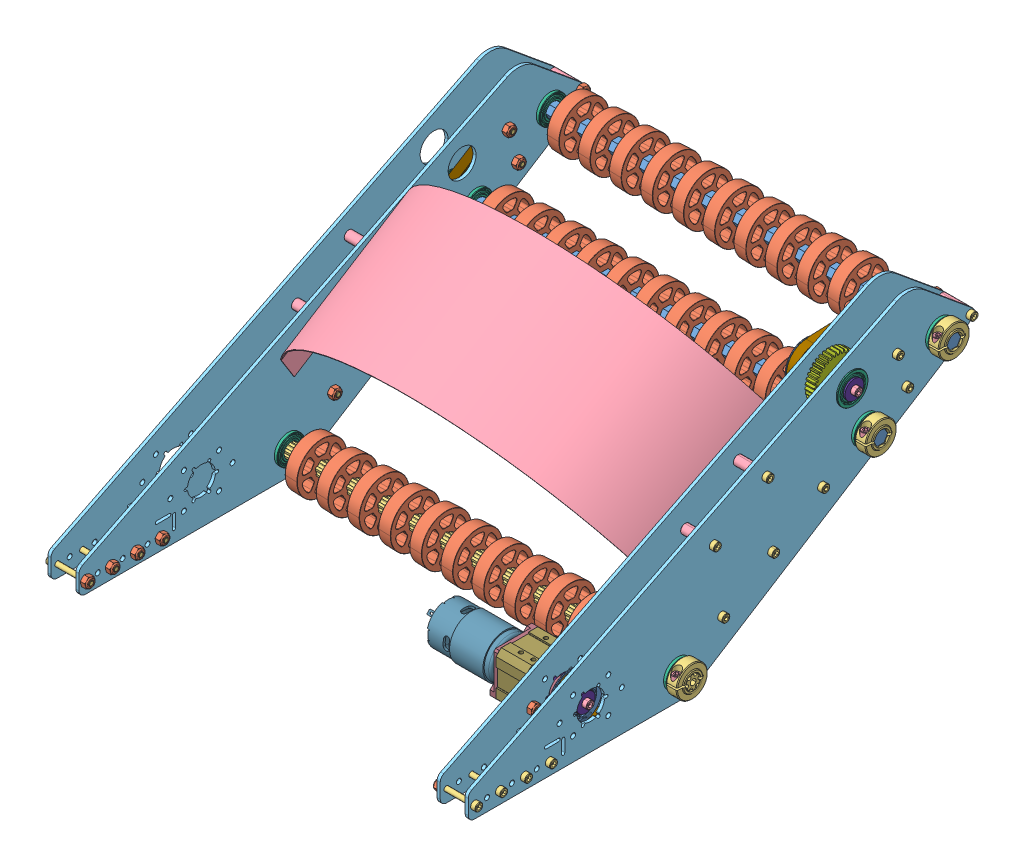
SolidWorks assembly am-4938 AndyMark Everybot Manipulator Assembly & mount, configuration Default. Lengths in mm.
Overall size (460.38 280.97 519.68).
230 component instances, 40 part files, 0 mates.
Components (placement in the parent):
- am-4938 AndyMark Everybot Manipulator Assembly.STEP-1: am-4938 AndyMark Everybot Manipulator Assembly.STEP [Default] at origin size (460.38 280.97 519.68)
  - 9mm wide 24T 500 Hex.STEP-1: 9mm wide 24T 500 Hex.STEP [Default] at (375.9591 173.9174 489.4692) x (1 0 0) z (0 0.018419 0.99983) size (14 42 42)
    - am-3403 24 tooth HTD pulley half 500hex.STEP-1: am-3403 24 tooth HTD pulley half 500hex.STEP [Default] at (-136.5229 43.891 78.8344) size (8.91 42 42)
    - am-3403 24 tooth HTD pulley half 500hex.STEP-2: am-3403 24 tooth HTD pulley half 500hex.STEP [Default] at (-136.5229 43.891 36.8344) x (-1 0 0) z (0 0 -1) size (8.91 42 42)
  - 9mm wide 24T 500 Hex.STEP-2: 9mm wide 24T 500 Hex.STEP [Default] at (351.0194 381.3222 230.4036) x (1 0 0) z (0 -0.838389 0.545072) size (14 42 42)
    - am-3403 24 tooth HTD pulley half 500hex.STEP-1: am-3403 24 tooth HTD pulley half 500hex.STEP [Default] at (-136.5229 43.891 78.8344) size (8.91 42 42)
    - am-3403 24 tooth HTD pulley half 500hex.STEP-2: am-3403 24 tooth HTD pulley half 500hex.STEP [Default] at (-136.5229 43.891 36.8344) x (-1 0 0) z (0 0 -1) size (8.91 42 42)
  - 9mm wide 24T 500 Hex.STEP-3: 9mm wide 24T 500 Hex.STEP [Default] at (349.4573 384.489 140.1259) x (1 0 0) z (0 -0.834137 0.551557) size (14 42 42)
    - am-3403 24 tooth HTD pulley half 500hex.STEP-1: am-3403 24 tooth HTD pulley half 500hex.STEP [Default] at (-136.5229 43.891 78.8344) size (8.91 42 42)
    - am-3403 24 tooth HTD pulley half 500hex.STEP-2: am-3403 24 tooth HTD pulley half 500hex.STEP [Default] at (-136.5229 43.891 36.8344) x (-1 0 0) z (0 0 -1) size (8.91 42 42)
  - 9mm wide 24T 500 Hex.STEP-4: 9mm wide 24T 500 Hex.STEP [Default] at (375.9591 191.0878 396.7517) x (1 0 0) z (0 -0.5 0.866025) size (14 42 42)
    - am-3403 24 tooth HTD pulley half 500hex.STEP-1: am-3403 24 tooth HTD pulley half 500hex.STEP [Default] at (-136.5229 43.891 78.8344) size (8.91 42 42)
    - am-3403 24 tooth HTD pulley half 500hex.STEP-2: am-3403 24 tooth HTD pulley half 500hex.STEP [Default] at (-136.5229 43.891 36.8344) x (-1 0 0) z (0 0 -1) size (8.91 42 42)
  - AndyMark Everybot Spacer Subassembly.STEP-1: AndyMark Everybot Spacer Subassembly.STEP [Default] at (54.6794 -110.646 280.1551) size (42.93 11.21 11.21)
    - 10-32 Nylock Nut 1_90631A411.STEP-1: 10-32 Nylock Nut 1_90631A411.STEP [Default] at (168.4198 387.9509 141.8561) x (0 1 0) z (0 0 1) size (9.55 5.96 11.02)
    - 10-32x1500_shcs_HX-SHCS 0.19-32x1.375x1-C.STEP-1: 10-32x1500_shcs_HX-SHCS 0.19-32x1.375x1-C.STEP [Default] at (204.9958 387.9509 141.8561) x (-1 0 0) z (0 -0.673367 0.739309) size (42.93 7.94 7.94)
    - am-3876 1000long .192ID Aluminum Spacer.STEP-1: am-3876 1000long .192ID Aluminum Spacer.STEP [Default] at (171.5948 387.9509 141.8561) x (0 -0.090635 0.995884) z (0 0.995884 0.090635) size (9.53 25.4 9.53)
  - AndyMark Everybot Spacer Subassembly.STEP-2: AndyMark Everybot Spacer Subassembly.STEP [Default] at (54.6794 -37.8081 18.3964) size (42.93 11.21 11.21)
    - 10-32 Nylock Nut 1_90631A411.STEP-1: 10-32 Nylock Nut 1_90631A411.STEP [Default] at (168.4198 387.9509 141.8561) x (0 1 0) z (0 0 1) size (9.55 5.96 11.02)
    - 10-32x1500_shcs_HX-SHCS 0.19-32x1.375x1-C.STEP-1: 10-32x1500_shcs_HX-SHCS 0.19-32x1.375x1-C.STEP [Default] at (204.9958 387.9509 141.8561) x (-1 0 0) z (0 -0.673367 0.739309) size (42.93 7.94 7.94)
    - am-3876 1000long .192ID Aluminum Spacer.STEP-1: am-3876 1000long .192ID Aluminum Spacer.STEP [Default] at (171.5948 387.9509 141.8561) x (0 -0.090635 0.995884) z (0 0.995884 0.090635) size (9.53 25.4 9.53)
  - AndyMark Everybot Spacer Subassembly.STEP-3: AndyMark Everybot Spacer Subassembly.STEP [Default] at (54.6794 -76.9148 226.3549) size (42.93 11.21 11.21)
    - 10-32 Nylock Nut 1_90631A411.STEP-1: 10-32 Nylock Nut 1_90631A411.STEP [Default] at (168.4198 387.9509 141.8561) x (0 1 0) z (0 0 1) size (9.55 5.96 11.02)
    - 10-32x1500_shcs_HX-SHCS 0.19-32x1.375x1-C.STEP-1: 10-32x1500_shcs_HX-SHCS 0.19-32x1.375x1-C.STEP [Default] at (204.9958 387.9509 141.8561) x (-1 0 0) z (0 -0.673367 0.739309) size (42.93 7.94 7.94)
    - am-3876 1000long .192ID Aluminum Spacer.STEP-1: am-3876 1000long .192ID Aluminum Spacer.STEP [Default] at (171.5948 387.9509 141.8561) x (0 -0.090635 0.995884) z (0 0.995884 0.090635) size (9.53 25.4 9.53)
  - AndyMark Everybot Spacer Subassembly.STEP-4: AndyMark Everybot Spacer Subassembly.STEP [Default] at (54.6794 144.8465 -39.0656) x (1 0 0) z (0 -0.832151 0.55455) size (42.93 11.21 11.21)
    - 10-32 Nylock Nut 1_90631A411.STEP-1: 10-32 Nylock Nut 1_90631A411.STEP [Default] at (168.4198 387.9509 141.8561) x (0 1 0) z (0 0 1) size (9.55 5.96 11.02)
    - 10-32x1500_shcs_HX-SHCS 0.19-32x1.375x1-C.STEP-1: 10-32x1500_shcs_HX-SHCS 0.19-32x1.375x1-C.STEP [Default] at (204.9958 387.9509 141.8561) x (-1 0 0) z (0 -0.673367 0.739309) size (42.93 7.94 7.94)
    - am-3876 1000long .192ID Aluminum Spacer.STEP-1: am-3876 1000long .192ID Aluminum Spacer.STEP [Default] at (171.5948 387.9509 141.8561) x (0 -0.090635 0.995884) z (0 0.995884 0.090635) size (9.53 25.4 9.53)
  - 57 Sport 4_1 with Flange Mount and 775.STEP-1: 57 Sport 4_1 with Flange Mount and 775.STEP [Default] at (512.1422 191.8089 396.7872) size (148.8 62.86 82.55)
    - am-XXXX - 57 Sport 500 Hex Output Plug.STEP-1: am-XXXX - 57 Sport 500 Hex Output Plug.STEP [Default] at (-295.3931 6.0609 150.085) x (0 0 -1) z (1 0 0) size (44.45 44.45 56.57)
      - am-XXXX - 57 Sport 500 Hex Shaft.STEP-1: am-XXXX - 57 Sport 500 Hex Shaft.STEP [Default] at (0 0 6.1595) x (0.145042 0.989426 0) z (0 0 1) size (14.67 12.71 56.57)
      - Output Block.STEP-1: Output Block.STEP [Default] at origin size (44.45 44.45 20.32)
      - retaining Ring 0500 - Mcm 98410A122_98410A122.STEP-1: retaining Ring 0500 - Mcm 98410A122_98410A122.STEP [Default] at (0 0 -14.5034) x (0 0 1) z (-0.999848 0.017452 0) size (0.89 16.1 14.34)
      - R8ZZ Bearing.STEP-1: R8ZZ Bearing.STEP [Default] at (0 0 6.1595) x (0 0 -1) z (0.975423 0.220339 0) size (7.94 28.57 28.57)
      - R8ZZ Bearing.STEP-2: R8ZZ Bearing.STEP [Default] at (0 0 -5.842) x (0 0 -1) z (0.99707 -0.076493 0) size (7.94 28.57 28.57)
    - am-XXXX - 4_1 Input Stage.STEP-1: am-XXXX - 4_1 Input Stage.STEP [Default] at (-312.8556 6.0609 150.085) x (0 -0.369103 0.929389) z (-1 0 0) size (35.15 35.15 14.63)
      - am-XXXX - 57 Sport Shaft Carrier Plate.STEP-1: am-XXXX - 57 Sport Shaft Carrier Plate.STEP [Default] at origin size (31.12 31.12 14.63)
      - 16T Planet Gear.STEP-1: 16T Planet Gear.STEP [Default] at (-11.8222 1.3023 11.8494) x (0 0 -1) z (1 0 0) size (7.09 12.42 12.42)
      - 16T Planet Gear.STEP-2: 16T Planet Gear.STEP [Default] at (1.3023 11.8222 11.8494) x (0 0 -1) z (0 -1 0) size (7.09 12.42 12.42)
      - 16T Planet Gear.STEP-3: 16T Planet Gear.STEP [Default] at (11.8222 -1.3023 11.8494) x (0 0 -1) z (-1 0 0) size (7.09 12.42 12.42)
      - 16T Planet Gear.STEP-4: 16T Planet Gear.STEP [Default] at (-1.3023 -11.8222 11.8494) x (0 0 -1) z (0 1 0) size (7.09 12.42 12.42)
    - am-4132 57 Sport Flange Mount.STEP-1: am-4132 57 Sport Flange Mount.STEP [Default] at (-295.3931 6.0609 150.085) x (0 0 1) z (0 1 0) size (82.55 6.35 47.62)
    - am-XXXX - 57 Sport 1 Stage Ring Gear Housing.STEP-1: am-XXXX - 57 Sport 1 Stage Ring Gear Housing.STEP [Default] at (-314.3161 6.0609 150.085) x (0 -1 0) z (1 0 0) size (47.63 47.63 31.5)
    - am-3765 - 57 Sport Motor Block.STEP-1: am-3765 - 57 Sport Motor Block.STEP [Default] at (-333.8741 6.0609 150.085) x (0 0 -1) z (1 0 0) size (44.45 44.45 8.89)
    - 775 RedLine.STEP-1: 775 RedLine.STEP [Default] at (-337.6841 6.0609 150.085) x (-1 0 0) z (0 0.707107 -0.707107) size (87.75 44.83 44.07)
    - M4 x .7mm x 8mm SHCS_91290A140.STEP-1: M4 x .7mm x 8mm SHCS_91290A140.STEP [Default] at (-341.9503 -4.1921 139.8319) x (0 -0.977065 0.212941) z (-1 0 0) size (7 7 12.01)
    - M4 Lock Washer_91169A160.STEP-1: M4 Lock Washer_91169A160.STEP [Default] at (-333.1503 -4.1921 139.8319) x (0 0.294925 0.95552) z (-1 0 0) size (7.6 7.6 1.68)
    - M4 x .7mm x 8mm SHCS_91290A140.STEP-2: M4 x .7mm x 8mm SHCS_91290A140.STEP [Default] at (-341.9503 16.314 160.338) x (0 -0.411961 0.911202) z (-1 0 0) size (7 7 12.01)
    - M4 Lock Washer_91169A160.STEP-2: M4 Lock Washer_91169A160.STEP [Default] at (-333.0699 16.314 160.338) x (0 -0.95552 -0.294925) z (1 0 0) size (7.6 7.6 1.68)
    - am-3784 - RS-700 Motor Pinion Gear.STEP-1: am-3784 - RS-700 Motor Pinion Gear.STEP [Default] at (-323.5158 4.9342 148.4301) size (11.94 12.42 12.42)
    - 10-32 x 1.750 SHCS_90128A953.STEP-1: 10-32 x 1.750 SHCS_90128A953.STEP [Default] at (-339.8431 24.0214 132.1245) x (0 0.297258 -0.954797) z (-1 0 0) size (7.92 7.92 49.28)
    - 10-32 x 1.750 SHCS_90128A953.STEP-2: 10-32 x 1.750 SHCS_90128A953.STEP [Default] at (-339.8431 -11.8996 168.0455) x (0 -0.297258 0.954797) z (-1 0 0) size (7.92 7.92 49.28)
    - Thrust washer - 775 Sport.STEP-1: Thrust washer - 775 Sport.STEP [Default] at (-329.01 6.0609 150.085) x (0 0 -1) z (1 0 0) size (31 31 1.52)
    - BHCS 10-32 x 0.500_91255A265.STEP-1: BHCS 10-32 x 0.500_91255A265.STEP [Default] at (-289.6527 24.0214 168.0455) x (0 0 -1) z (1 0 0) size (9.17 9.17 15.27)
    - BHCS 10-32 x 0.500_91255A265.STEP-2: BHCS 10-32 x 0.500_91255A265.STEP [Default] at (-289.6527 -11.8996 132.1245) x (0 0 -1) z (1 0 0) size (9.17 9.17 15.27)
  - am-1526 500Hex Collar Clamp.STEP-1: am-1526 500Hex Collar Clamp.STEP [Default] at (238.9418 338.5749 286.0754) x (0 0.052851 0.998602) z (-1 0 0) size (31.72 31.75 12.7)
    - 500Hex Collar Clamp Body.STEP-1: 500Hex Collar Clamp Body.STEP [Default] at (-94.2794 15.3021 33.01) size (31.72 31.75 12.7)
    - 10-32x0500_shcs_HX-SHCS 0.19-32x1.375x1-C.STEP-1: 10-32x0500_shcs_HX-SHCS 0.19-32x1.375x1-C.STEP [Default] at (-83.1669 24.3191 39.36) x (0 -1 0) z (0 0 1) size (17.53 7.94 7.94)
  - am-1526 500Hex Collar Clamp.STEP-2: am-1526 500Hex Collar Clamp.STEP [Default] at (303.7214 290.7812 360.5945) x (0 0.052851 0.998602) z (-1 0 0) size (31.72 31.75 12.7)
    - 500Hex Collar Clamp Body.STEP-1: 500Hex Collar Clamp Body.STEP [Default] at (-94.2794 15.3021 33.01) size (31.72 31.75 12.7)
    - 10-32x0500_shcs_HX-SHCS 0.19-32x1.375x1-C.STEP-1: 10-32x0500_shcs_HX-SHCS 0.19-32x1.375x1-C.STEP [Default] at (-83.1669 24.3191 39.36) x (0 -1 0) z (0 0 1) size (17.53 7.94 7.94)
  - am-1526 500Hex Collar Clamp.STEP-3: am-1526 500Hex Collar Clamp.STEP [Default] at (303.7214 330.6759 284.8827) x (0 -0.030782 0.999526) z (-1 0 0) size (31.72 31.75 12.7)
    - 500Hex Collar Clamp Body.STEP-1: 500Hex Collar Clamp Body.STEP [Default] at (-94.2794 15.3021 33.01) size (31.72 31.75 12.7)
    - 10-32x0500_shcs_HX-SHCS 0.19-32x1.375x1-C.STEP-1: 10-32x0500_shcs_HX-SHCS 0.19-32x1.375x1-C.STEP [Default] at (-83.1669 24.3191 39.36) x (0 -1 0) z (0 0 1) size (17.53 7.94 7.94)
  - am-1526 500Hex Collar Clamp.STEP-4: am-1526 500Hex Collar Clamp.STEP [Default] at (303.7214 171.6969 553.2396) x (0 0.052851 0.998602) z (-1 0 0) size (31.72 31.75 12.7)
    - 500Hex Collar Clamp Body.STEP-1: 500Hex Collar Clamp Body.STEP [Default] at (-94.2794 15.3021 33.01) size (31.72 31.75 12.7)
    - 10-32x0500_shcs_HX-SHCS 0.19-32x1.375x1-C.STEP-1: 10-32x0500_shcs_HX-SHCS 0.19-32x1.375x1-C.STEP [Default] at (-83.1669 24.3191 39.36) x (0 -1 0) z (0 0 1) size (17.53 7.94 7.94)
  - AndyMark Everybot Spacer Subassembly.STEP-5: AndyMark Everybot Spacer Subassembly.STEP [Default] at (26.3939 261.0166 834.7627) x (-1 0 0) z (0 -0.924911 -0.380184) size (42.93 11.21 11.21)
    - 10-32 Nylock Nut 1_90631A411.STEP-1: 10-32 Nylock Nut 1_90631A411.STEP [Default] at (168.4198 387.9509 141.8561) x (0 1 0) z (0 0 1) size (9.55 5.96 11.02)
    - 10-32x1500_shcs_HX-SHCS 0.19-32x1.375x1-C.STEP-1: 10-32x1500_shcs_HX-SHCS 0.19-32x1.375x1-C.STEP [Default] at (204.9958 387.9509 141.8561) x (-1 0 0) z (0 -0.673367 0.739309) size (42.93 7.94 7.94)
    - am-3876 1000long .192ID Aluminum Spacer.STEP-1: am-3876 1000long .192ID Aluminum Spacer.STEP [Default] at (171.5948 387.9509 141.8561) x (0 -0.090635 0.995884) z (0 0.995884 0.090635) size (9.53 25.4 9.53)
  - AndyMark Everybot Spacer Subassembly.STEP-6: AndyMark Everybot Spacer Subassembly.STEP [Default] at (26.3939 294.7478 780.9625) x (-1 0 0) z (0 -0.924911 -0.380184) size (42.93 11.21 11.21)
    - 10-32 Nylock Nut 1_90631A411.STEP-1: 10-32 Nylock Nut 1_90631A411.STEP [Default] at (168.4198 387.9509 141.8561) x (0 1 0) z (0 0 1) size (9.55 5.96 11.02)
    - 10-32x1500_shcs_HX-SHCS 0.19-32x1.375x1-C.STEP-1: 10-32x1500_shcs_HX-SHCS 0.19-32x1.375x1-C.STEP [Default] at (204.9958 387.9509 141.8561) x (-1 0 0) z (0 -0.673367 0.739309) size (42.93 7.94 7.94)
    - am-3876 1000long .192ID Aluminum Spacer.STEP-1: am-3876 1000long .192ID Aluminum Spacer.STEP [Default] at (171.5948 387.9509 141.8561) x (0 -0.090635 0.995884) z (0 0.995884 0.090635) size (9.53 25.4 9.53)
  - AndyMark Everybot Spacer Subassembly.STEP-7: AndyMark Everybot Spacer Subassembly.STEP [Default] at (26.3939 225.6505 775.1858) x (-1 0 0) z (0 -0.924911 -0.380184) size (42.93 11.21 11.21)
    - 10-32 Nylock Nut 1_90631A411.STEP-1: 10-32 Nylock Nut 1_90631A411.STEP [Default] at (168.4198 387.9509 141.8561) x (0 1 0) z (0 0 1) size (9.55 5.96 11.02)
    - 10-32x1500_shcs_HX-SHCS 0.19-32x1.375x1-C.STEP-1: 10-32x1500_shcs_HX-SHCS 0.19-32x1.375x1-C.STEP [Default] at (204.9958 387.9509 141.8561) x (-1 0 0) z (0 -0.673367 0.739309) size (42.93 7.94 7.94)
    - am-3876 1000long .192ID Aluminum Spacer.STEP-1: am-3876 1000long .192ID Aluminum Spacer.STEP [Default] at (171.5948 387.9509 141.8561) x (0 -0.090635 0.995884) z (0 0.995884 0.090635) size (9.53 25.4 9.53)
  - AndyMark Everybot Spacer Subassembly.STEP-8: AndyMark Everybot Spacer Subassembly.STEP [Default] at (26.3939 333.8545 573.004) x (-1 0 0) z (0 -0.924911 -0.380184) size (42.93 11.21 11.21)
    - 10-32 Nylock Nut 1_90631A411.STEP-1: 10-32 Nylock Nut 1_90631A411.STEP [Default] at (168.4198 387.9509 141.8561) x (0 1 0) z (0 0 1) size (9.55 5.96 11.02)
    - 10-32x1500_shcs_HX-SHCS 0.19-32x1.375x1-C.STEP-1: 10-32x1500_shcs_HX-SHCS 0.19-32x1.375x1-C.STEP [Default] at (204.9958 387.9509 141.8561) x (-1 0 0) z (0 -0.673367 0.739309) size (42.93 7.94 7.94)
    - am-3876 1000long .192ID Aluminum Spacer.STEP-1: am-3876 1000long .192ID Aluminum Spacer.STEP [Default] at (171.5948 387.9509 141.8561) x (0 -0.090635 0.995884) z (0 0.995884 0.090635) size (9.53 25.4 9.53)
  - am-1526 500Hex Collar Clamp.STEP-5: am-1526 500Hex Collar Clamp.STEP [Default] at (-143.9282 338.5749 286.0754) x (0 0.052851 0.998602) z (-1 0 0) size (31.72 31.75 12.7)
    - 500Hex Collar Clamp Body.STEP-1: 500Hex Collar Clamp Body.STEP [Default] at (-94.2794 15.3021 33.01) size (31.72 31.75 12.7)
    - 10-32x0500_shcs_HX-SHCS 0.19-32x1.375x1-C.STEP-1: 10-32x0500_shcs_HX-SHCS 0.19-32x1.375x1-C.STEP [Default] at (-83.1669 24.3191 39.36) x (0 -1 0) z (0 0 1) size (17.53 7.94 7.94)
  - am-1526 500Hex Collar Clamp.STEP-6: am-1526 500Hex Collar Clamp.STEP [Default] at (-143.9282 291.5849 361.5416) x (0 0.052851 0.998602) z (-1 0 0) size (31.72 31.75 12.7)
    - 500Hex Collar Clamp Body.STEP-1: 500Hex Collar Clamp Body.STEP [Default] at (-94.2794 15.3021 33.01) size (31.72 31.75 12.7)
    - 10-32x0500_shcs_HX-SHCS 0.19-32x1.375x1-C.STEP-1: 10-32x0500_shcs_HX-SHCS 0.19-32x1.375x1-C.STEP [Default] at (-83.1669 24.3191 39.36) x (0 -1 0) z (0 0 1) size (17.53 7.94 7.94)
  - am-1526 500Hex Collar Clamp.STEP-7: am-1526 500Hex Collar Clamp.STEP [Default] at (-143.9282 171.6969 553.2396) x (0 0.052851 0.998602) z (-1 0 0) size (31.72 31.75 12.7)
    - 500Hex Collar Clamp Body.STEP-1: 500Hex Collar Clamp Body.STEP [Default] at (-94.2794 15.3021 33.01) size (31.72 31.75 12.7)
    - 10-32x0500_shcs_HX-SHCS 0.19-32x1.375x1-C.STEP-1: 10-32x0500_shcs_HX-SHCS 0.19-32x1.375x1-C.STEP [Default] at (-83.1669 24.3191 39.36) x (0 -1 0) z (0 0 1) size (17.53 7.94 7.94)
  - 9mm wide 24T 500 Hex.STEP-5: 9mm wide 24T 500 Hex.STEP [Default] at (-22.0558 172.1698 396.8644) x (1 0 0) z (0 -0.216531 0.976276) size (14 42 42)
    - am-3403 24 tooth HTD pulley half 500hex.STEP-1: am-3403 24 tooth HTD pulley half 500hex.STEP [Default] at (-136.5229 43.891 78.8344) size (8.91 42 42)
    - am-3403 24 tooth HTD pulley half 500hex.STEP-2: am-3403 24 tooth HTD pulley half 500hex.STEP [Default] at (-136.5229 43.891 36.8344) x (-1 0 0) z (0 0 -1) size (8.91 42 42)
  - 9mm wide 24T 500 Hex.STEP-6: 9mm wide 24T 500 Hex.STEP [Default] at (-22.0558 323.6557 134.2603) x (1 0 0) z (0 0.040546 0.999178) size (14 42 42)
    - am-3403 24 tooth HTD pulley half 500hex.STEP-1: am-3403 24 tooth HTD pulley half 500hex.STEP [Default] at (-136.5229 43.891 78.8344) size (8.91 42 42)
    - am-3403 24 tooth HTD pulley half 500hex.STEP-2: am-3403 24 tooth HTD pulley half 500hex.STEP [Default] at (-136.5229 43.891 36.8344) x (-1 0 0) z (0 0 -1) size (8.91 42 42)
  - AndyMark Everybot Spacer Subassembly.STEP-9: AndyMark Everybot Spacer Subassembly.STEP [Default] at (26.3939 336.767 648.1233) x (-1 0 0) z (0 -0.924911 -0.380184) size (42.93 11.21 11.21)
    - 10-32 Nylock Nut 1_90631A411.STEP-1: 10-32 Nylock Nut 1_90631A411.STEP [Default] at (168.4198 387.9509 141.8561) x (0 1 0) z (0 0 1) size (9.55 5.96 11.02)
    - 10-32x1500_shcs_HX-SHCS 0.19-32x1.375x1-C.STEP-1: 10-32x1500_shcs_HX-SHCS 0.19-32x1.375x1-C.STEP [Default] at (204.9958 387.9509 141.8561) x (-1 0 0) z (0 -0.673367 0.739309) size (42.93 7.94 7.94)
    - am-3876 1000long .192ID Aluminum Spacer.STEP-1: am-3876 1000long .192ID Aluminum Spacer.STEP [Default] at (171.5948 387.9509 141.8561) x (0 -0.090635 0.995884) z (0 0.995884 0.090635) size (9.53 25.4 9.53)
  - AndyMark Everybot Spacer Subassembly.STEP-10: AndyMark Everybot Spacer Subassembly.STEP [Default] at (26.3939 303.189 638.5172) x (-1 0 0) z (0 -0.924911 -0.380184) size (42.93 11.21 11.21)
    - 10-32 Nylock Nut 1_90631A411.STEP-1: 10-32 Nylock Nut 1_90631A411.STEP [Default] at (168.4198 387.9509 141.8561) x (0 1 0) z (0 0 1) size (9.55 5.96 11.02)
    - 10-32x1500_shcs_HX-SHCS 0.19-32x1.375x1-C.STEP-1: 10-32x1500_shcs_HX-SHCS 0.19-32x1.375x1-C.STEP [Default] at (204.9958 387.9509 141.8561) x (-1 0 0) z (0 -0.673367 0.739309) size (42.93 7.94 7.94)
    - am-3876 1000long .192ID Aluminum Spacer.STEP-1: am-3876 1000long .192ID Aluminum Spacer.STEP [Default] at (171.5948 387.9509 141.8561) x (0 -0.090635 0.995884) z (0 0.995884 0.090635) size (9.53 25.4 9.53)
  - AndyMark Everybot Spacer Subassembly.STEP-11: AndyMark Everybot Spacer Subassembly.STEP [Default] at (26.3939 256.8115 724.2868) x (-1 0 0) z (0 -0.924307 -0.38165) size (42.93 11.21 11.21)
    - 10-32 Nylock Nut 1_90631A411.STEP-1: 10-32 Nylock Nut 1_90631A411.STEP [Default] at (168.4198 387.9509 141.8561) x (0 1 0) z (0 0 1) size (9.55 5.96 11.02)
    - 10-32x1500_shcs_HX-SHCS 0.19-32x1.375x1-C.STEP-1: 10-32x1500_shcs_HX-SHCS 0.19-32x1.375x1-C.STEP [Default] at (204.9958 387.9509 141.8561) x (-1 0 0) z (0 -0.673367 0.739309) size (42.93 7.94 7.94)
    - am-3876 1000long .192ID Aluminum Spacer.STEP-1: am-3876 1000long .192ID Aluminum Spacer.STEP [Default] at (171.5948 387.9509 141.8561) x (0 -0.090635 0.995884) z (0 0.995884 0.090635) size (9.53 25.4 9.53)
  - AndyMark Everybot Spacer Subassembly.STEP-12: AndyMark Everybot Spacer Subassembly.STEP [Default] at (26.3939 193.7876 826.1337) x (-1 0 0) z (0 -0.924911 -0.380184) size (42.93 11.21 11.21)
    - 10-32 Nylock Nut 1_90631A411.STEP-1: 10-32 Nylock Nut 1_90631A411.STEP [Default] at (168.4198 387.9509 141.8561) x (0 1 0) z (0 0 1) size (9.55 5.96 11.02)
    - 10-32x1500_shcs_HX-SHCS 0.19-32x1.375x1-C.STEP-1: 10-32x1500_shcs_HX-SHCS 0.19-32x1.375x1-C.STEP [Default] at (204.9958 387.9509 141.8561) x (-1 0 0) z (0 -0.673367 0.739309) size (42.93 7.94 7.94)
    - am-3876 1000long .192ID Aluminum Spacer.STEP-1: am-3876 1000long .192ID Aluminum Spacer.STEP [Default] at (171.5948 387.9509 141.8561) x (0 -0.090635 0.995884) z (0 0.995884 0.090635) size (9.53 25.4 9.53)
  - AndyMark Everybot Spacer Subassembly.STEP-13: AndyMark Everybot Spacer Subassembly.STEP [Default] at (54.6794 509.1158 698.3459) x (1 0 0) z (0 0.399295 -0.916823) size (42.93 11.21 11.21)
    - 10-32 Nylock Nut 1_90631A411.STEP-1: 10-32 Nylock Nut 1_90631A411.STEP [Default] at (168.4198 387.9509 141.8561) x (0 1 0) z (0 0 1) size (9.55 5.96 11.02)
    - 10-32x1500_shcs_HX-SHCS 0.19-32x1.375x1-C.STEP-1: 10-32x1500_shcs_HX-SHCS 0.19-32x1.375x1-C.STEP [Default] at (204.9958 387.9509 141.8561) x (-1 0 0) z (0 -0.673367 0.739309) size (42.93 7.94 7.94)
    - am-3876 1000long .192ID Aluminum Spacer.STEP-1: am-3876 1000long .192ID Aluminum Spacer.STEP [Default] at (171.5948 387.9509 141.8561) x (0 -0.090635 0.995884) z (0 0.995884 0.090635) size (9.53 25.4 9.53)
  - AndyMark Everybot Spacer Subassembly.STEP-14: AndyMark Everybot Spacer Subassembly.STEP [Default] at (54.6794 618.5172 510.7294) x (1 0 0) z (0 0.399295 -0.916823) size (42.93 11.21 11.21)
    - 10-32 Nylock Nut 1_90631A411.STEP-1: 10-32 Nylock Nut 1_90631A411.STEP [Default] at (168.4198 387.9509 141.8561) x (0 1 0) z (0 0 1) size (9.55 5.96 11.02)
    - 10-32x1500_shcs_HX-SHCS 0.19-32x1.375x1-C.STEP-1: 10-32x1500_shcs_HX-SHCS 0.19-32x1.375x1-C.STEP [Default] at (204.9958 387.9509 141.8561) x (-1 0 0) z (0 -0.673367 0.739309) size (42.93 7.94 7.94)
    - am-3876 1000long .192ID Aluminum Spacer.STEP-1: am-3876 1000long .192ID Aluminum Spacer.STEP [Default] at (171.5948 387.9509 141.8561) x (0 -0.090635 0.995884) z (0 0.995884 0.090635) size (9.53 25.4 9.53)
  - AndyMark Everybot Spacer Subassembly.STEP-15: AndyMark Everybot Spacer Subassembly.STEP [Default] at (54.6794 572.7943 596.5254) x (1 0 0) z (0 0.399295 -0.916823) size (42.93 11.21 11.21)
    - 10-32 Nylock Nut 1_90631A411.STEP-1: 10-32 Nylock Nut 1_90631A411.STEP [Default] at (168.4198 387.9509 141.8561) x (0 1 0) z (0 0 1) size (9.55 5.96 11.02)
    - 10-32x1500_shcs_HX-SHCS 0.19-32x1.375x1-C.STEP-1: 10-32x1500_shcs_HX-SHCS 0.19-32x1.375x1-C.STEP [Default] at (204.9958 387.9509 141.8561) x (-1 0 0) z (0 -0.673367 0.739309) size (42.93 7.94 7.94)
    - am-3876 1000long .192ID Aluminum Spacer.STEP-1: am-3876 1000long .192ID Aluminum Spacer.STEP [Default] at (171.5948 387.9509 141.8561) x (0 -0.090635 0.995884) z (0 0.995884 0.090635) size (9.53 25.4 9.53)
  - AndyMark Everybot Spacer Subassembly.STEP-16: AndyMark Everybot Spacer Subassembly.STEP [Default] at (54.6794 652.0951 520.3355) x (1 0 0) z (0 0.399295 -0.916823) size (42.93 11.21 11.21)
    - 10-32 Nylock Nut 1_90631A411.STEP-1: 10-32 Nylock Nut 1_90631A411.STEP [Default] at (168.4198 387.9509 141.8561) x (0 1 0) z (0 0 1) size (9.55 5.96 11.02)
    - 10-32x1500_shcs_HX-SHCS 0.19-32x1.375x1-C.STEP-1: 10-32x1500_shcs_HX-SHCS 0.19-32x1.375x1-C.STEP [Default] at (204.9958 387.9509 141.8561) x (-1 0 0) z (0 -0.673367 0.739309) size (42.93 7.94 7.94)
    - am-3876 1000long .192ID Aluminum Spacer.STEP-1: am-3876 1000long .192ID Aluminum Spacer.STEP [Default] at (171.5948 387.9509 141.8561) x (0 -0.090635 0.995884) z (0 0.995884 0.090635) size (9.53 25.4 9.53)
  - am-4938_in-plate AndyMark EveryBot Intake Plate_V2.STEP-1: am-4938_in-plate AndyMark EveryBot Intake Plate_V2.STEP [Default] at (254.8492 156.5948 671.6871) size (3.17 244.43 516.2)
  - am-4938_in-plate AndyMark EveryBot Intake Plate_V2.STEP-2: am-4938_in-plate AndyMark EveryBot Intake Plate_V2.STEP [Default] at (226.2742 156.5948 671.6871) size (3.17 244.43 516.2)
  - am-2986 FR8ZZ Hex Bearing.STEP-1: am-2986 FR8ZZ Hex Bearing.STEP [Default] at (256.4494 345.3116 281.1191) x (0 -0.052851 -0.998602) z (0 -0.998602 0.052851) size (31.12 7.94 31.12)
  - am-2986 FR8ZZ Hex Bearing.STEP-2: am-2986 FR8ZZ Hex Bearing.STEP [Default] at (221.499 345.3116 281.1191) x (0 0.838389 -0.545072) z (0 0.545072 0.838389) size (31.12 7.94 31.12)
  - am-4709 36T 20DP 500hex 375 FW.STEP-1: am-4709 36T 20DP 500hex 375 FW.STEP [Default] at (231.024 345.3116 281.1191) x (1 0 0) z (0 0.891241 0.453531) size (12.7 48.15 48.15)
  - am-3948-250 500H x 250IN Spacer.STEP-1: am-3948-250 500H x 250IN Spacer.STEP [Default] at (248.4865 345.3116 281.1191) x (0 0.052851 0.998602) z (-1 0 0) size (20 20 6.35)
  - am-4902 60T 5mm HTD Belt 9mm Wide.STEP-1: am-4902 60T 5mm HTD Belt 9mm Wide.STEP [Default] at (208.9344 345.3144 281.0487) x (1 0 0) z (0 -0.039538 0.999218) size (9 41.68 131.68)
  - am-4902 60T 5mm HTD Belt 9mm Wide.STEP-2: am-4902 60T 5mm HTD Belt 9mm Wide.STEP [Default] at (235.4362 197.8698 546.8722) x (1 0 0) z (0 0.176389 0.984321) size (9 41.68 131.68)
  - am-1692 2 in. Long 0.5 in OD F-F Steel Standoff_92230A135.STEP-1: am-1692 2 in. Long 0.5 in OD F-F Steel Standoff_92230A135.STEP [Default] at (231.0494 345.3116 281.1191) x (0 -0.453531 0.891241) z (1 0 0) size (14.71 14.77 59.16)
  - am-3948-063 500H x 063IN Spacer.STEP-1: am-3948-063 500H x 063IN Spacer.STEP [Default] at (206.0278 345.3116 281.1191) x (0 0.891241 0.453531) z (1 0 0) size (20 20 1.59)
  - 10-32x0500_shcs_HX-SHCS 0.19-32x1.375x1-C.STEP-1: 10-32x0500_shcs_HX-SHCS 0.19-32x1.375x1-C.STEP [Default] at (199.6143 345.3116 281.1191) x (1 0 0) z (0 0.014609 0.999893) size (17.53 7.94 7.94)
  - 10-32 Nylock Nut 1_90631A411.STEP-1: 10-32 Nylock Nut 1_90631A411.STEP [Default] at (226.2742 197.8698 515.1222) x (0 0.902435 0.430825) z (0 0.430825 -0.902435) size (9.55 5.96 11.02)
  - 10-32 Nylock Nut 1_90631A411.STEP-2: 10-32 Nylock Nut 1_90631A411.STEP [Default] at (226.2742 197.8698 578.6222) x (0 0.845049 0.534689) z (0 0.534689 -0.845049) size (9.55 5.96 11.02)
  - 10-32x750_shcs_90128A945.STEP-1: 10-32x750_shcs_90128A945.STEP [Default] at (235.7992 197.8698 515.1222) x (0 -0.644782 -0.764367) z (1 0 0) size (7.92 7.92 23.88)
  - 10-32x750_shcs_90128A945.STEP-2: 10-32x750_shcs_90128A945.STEP [Default] at (235.7992 197.8698 578.6222) x (0 0 -1) z (1 0 0) size (7.92 7.92 23.88)
  - am-3948-375 500H x 375IN Spacer.STEP-1: am-3948-375 500H x 375IN Spacer.STEP [Default] at (232.4337 197.8698 546.8722) x (0 0.091272 -0.995826) z (-1 0 0) size (20 20 9.53)
  - am-3948-063 500H x 063IN Spacer.STEP-2: am-3948-063 500H x 063IN Spacer.STEP [Default] at (248.0261 197.8698 546.8722) x (0 0.620323 0.784347) z (-1 0 0) size (20 20 1.59)
  - am-2986 FR8ZZ Hex Bearing.STEP-3: am-2986 FR8ZZ Hex Bearing.STEP [Default] at (227.8744 348.8728 191.1191) x (0 -0.052851 -0.998602) z (0 -0.998602 0.052851) size (31.12 7.94 31.12)
  - am-2986 FR8ZZ Hex Bearing.STEP-4: am-2986 FR8ZZ Hex Bearing.STEP [Default] at (250.074 348.8728 191.1191) x (0 0.902752 0.430162) z (0 -0.430162 0.902752) size (31.12 7.94 31.12)
  - am-3948-375 500H x 375IN Spacer.STEP-2: am-3948-375 500H x 375IN Spacer.STEP [Default] at (227.849 348.8728 191.1191) x (0 0.091272 0.995826) z (1 0 0) size (20 20 9.53)
  - am-3948-375 500H x 375IN Spacer.STEP-3: am-3948-375 500H x 375IN Spacer.STEP [Default] at (250.0994 301.8828 266.5853) x (0 0.091272 -0.995826) z (-1 0 0) size (20 20 9.53)
  - am-4709 36T 20DP 500hex 375 FW.STEP-2: am-4709 36T 20DP 500hex 375 FW.STEP [Default] at (229.4619 301.8828 266.5853) x (1 0 0) z (0 0.813642 0.581366) size (12.7 48.15 48.15)
  - am-2986 FR8ZZ Hex Bearing.STEP-5: am-2986 FR8ZZ Hex Bearing.STEP [Default] at (250.074 301.8828 266.5853) x (0 0.902752 0.430162) z (0 -0.430162 0.902752) size (31.12 7.94 31.12)
  - am-2986 FR8ZZ Hex Bearing.STEP-6: am-2986 FR8ZZ Hex Bearing.STEP [Default] at (227.8744 301.8828 266.5853) x (0 -0.052851 -0.998602) z (0 -0.998602 0.052851) size (31.12 7.94 31.12)
  - am-3948-500 500H x 500IN Spacer.STEP-1: am-3948-500 500H x 500IN Spacer.STEP [Default] at (250.074 348.8728 191.1191) x (0 0 1) z (-1 0 0) size (20 20 12.7)
  - am-2986 FR8ZZ Hex Bearing.STEP-7: am-2986 FR8ZZ Hex Bearing.STEP [Default] at (250.074 181.9948 458.2833) x (0 1 0) z (0 0 1) size (31.12 7.94 31.12)
  - am-2986 FR8ZZ Hex Bearing.STEP-8: am-2986 FR8ZZ Hex Bearing.STEP [Default] at (227.8744 181.9948 458.2833) x (0 0.381849 -0.924225) z (0 -0.924225 -0.381849) size (31.12 7.94 31.12)
  - am-3948-188 500H x 188IN Spacer.STEP-1: am-3948-188 500H x 188IN Spacer.STEP [Default] at (227.8744 181.9948 458.2833) x (0 -0.039215 -0.999231) z (1 0 0) size (20 20 4.78)
  - am-3948-125 500H x 125IN Spacer.STEP-1: am-3948-125 500H x 125IN Spacer.STEP [Default] at (246.899 181.9948 458.2833) x (0 -0.062923 0.998018) z (1 0 0) size (20 20 3.17)
  - am-1523 10 Fender Washer.STEP-1: am-1523 10 Fender Washer.STEP [Default] at (204.4403 345.3116 281.1191) x (0 -1 0) z (0 0 1) size (19.05 1.59 19.05)
  - am-1523 10 Fender Washer.STEP-2: am-1523 10 Fender Washer.STEP [Default] at (256.4494 345.3116 281.1191) x (0 -0.381849 0.924225) z (0 0.924225 0.381849) size (19.05 1.59 19.05)
  - 10-32x0500_shcs_HX-SHCS 0.19-32x1.375x1-C.STEP-2: 10-32x0500_shcs_HX-SHCS 0.19-32x1.375x1-C.STEP [Default] at (262.8629 345.3116 281.1191) x (-1 0 0) z (0 -0.924225 -0.381849) size (17.53 7.94 7.94)
  - am-1523 10 Fender Washer.STEP-3: am-1523 10 Fender Washer.STEP [Default] at (248.3087 197.8698 546.8722) x (0 -0.381849 0.924225) z (0 0.924225 0.381849) size (19.05 1.59 19.05)
  - 10-32x0500_shcs_HX-SHCS 0.19-32x1.375x1-C.STEP-3: 10-32x0500_shcs_HX-SHCS 0.19-32x1.375x1-C.STEP [Default] at (254.7222 197.8698 546.8722) x (-1 0 0) z (0 -0.924225 -0.381849) size (17.53 7.94 7.94)
  - 10-32x1500_shcs_HX-SHCS 0.19-32x1.375x1-C.STEP-1: 10-32x1500_shcs_HX-SHCS 0.19-32x1.375x1-C.STEP [Default] at (259.6752 169.2948 589.1371) x (-1 0 0) z (0 -0.673367 0.739309) size (42.93 7.94 7.94)
  - 10-32x1500_shcs_HX-SHCS 0.19-32x1.375x1-C.STEP-2: 10-32x1500_shcs_HX-SHCS 0.19-32x1.375x1-C.STEP [Default] at (259.6752 169.2948 614.5371) x (-1 0 0) z (0 -0.673367 0.739309) size (42.93 7.94 7.94)
  - 10-32x1500_shcs_HX-SHCS 0.19-32x1.375x1-C.STEP-3: 10-32x1500_shcs_HX-SHCS 0.19-32x1.375x1-C.STEP [Default] at (259.6752 169.2948 639.9371) x (-1 0 0) z (0 -0.673367 0.739309) size (42.93 7.94 7.94)
  - 10-32x1500_shcs_HX-SHCS 0.19-32x1.375x1-C.STEP-4: 10-32x1500_shcs_HX-SHCS 0.19-32x1.375x1-C.STEP [Default] at (259.6752 169.2948 665.3371) x (-1 0 0) z (0 -0.673367 0.739309) size (42.93 7.94 7.94)
  - 10-32 Nylock Nut 1_90631A411.STEP-3: 10-32 Nylock Nut 1_90631A411.STEP [Default] at (223.0992 169.2948 589.1371) x (0 0.488303 0.872674) z (0 -0.872674 0.488303) size (9.55 5.96 11.02)
  - 10-32 Nylock Nut 1_90631A411.STEP-4: 10-32 Nylock Nut 1_90631A411.STEP [Default] at (223.0992 169.2948 614.5371) x (0 0.488303 0.872674) z (0 -0.872674 0.488303) size (9.55 5.96 11.02)
  - 10-32 Nylock Nut 1_90631A411.STEP-5: 10-32 Nylock Nut 1_90631A411.STEP [Default] at (223.0992 169.2948 639.9371) x (0 0.488303 0.872674) z (0 -0.872674 0.488303) size (9.55 5.96 11.02)
  - 10-32 Nylock Nut 1_90631A411.STEP-6: 10-32 Nylock Nut 1_90631A411.STEP [Default] at (223.0992 169.2948 665.3371) x (0 0.488303 0.872674) z (0 -0.872674 0.488303) size (9.55 5.96 11.02)
  - am-4938_in-plate AndyMark EveryBot Intake Plate_V2.STEP-3: am-4938_in-plate AndyMark EveryBot Intake Plate_V2.STEP [Default] at (-142.0258 156.5948 671.6871) size (3.17 244.43 516.2)
  - am-4938_in-plate AndyMark EveryBot Intake Plate_V2.STEP-4: am-4938_in-plate AndyMark EveryBot Intake Plate_V2.STEP [Default] at (-170.6008 156.5948 671.6871) size (3.17 244.43 516.2)
  - 10-32x1500_shcs_HX-SHCS 0.19-32x1.375x1-C.STEP-5: 10-32x1500_shcs_HX-SHCS 0.19-32x1.375x1-C.STEP [Default] at (-178.6018 169.2948 665.3371) x (1 0 0) z (0 0.940412 -0.340038) size (42.93 7.94 7.94)
  - 10-32x1500_shcs_HX-SHCS 0.19-32x1.375x1-C.STEP-6: 10-32x1500_shcs_HX-SHCS 0.19-32x1.375x1-C.STEP [Default] at (-178.6018 169.2948 639.9371) x (1 0 0) z (0 0.940412 -0.340038) size (42.93 7.94 7.94)
  - 10-32x1500_shcs_HX-SHCS 0.19-32x1.375x1-C.STEP-7: 10-32x1500_shcs_HX-SHCS 0.19-32x1.375x1-C.STEP [Default] at (-178.6018 169.2948 614.5371) x (1 0 0) z (0 0.940412 -0.340038) size (42.93 7.94 7.94)
  - 10-32x1500_shcs_HX-SHCS 0.19-32x1.375x1-C.STEP-8: 10-32x1500_shcs_HX-SHCS 0.19-32x1.375x1-C.STEP [Default] at (-178.6018 169.2948 589.1371) x (1 0 0) z (0 0.940412 -0.340038) size (42.93 7.94 7.94)
  - am-2986 FR8ZZ Hex Bearing.STEP-9: am-2986 FR8ZZ Hex Bearing.STEP [Default] at (-146.801 348.8728 191.1191) x (0 0.902752 0.430162) z (0 -0.430162 0.902752) size (31.12 7.94 31.12)
  - am-2986 FR8ZZ Hex Bearing.STEP-10: am-2986 FR8ZZ Hex Bearing.STEP [Default] at (-169.0006 348.8728 191.1191) x (0 -0.052851 -0.998602) z (0 -0.998602 0.052851) size (31.12 7.94 31.12)
  - am-2986 FR8ZZ Hex Bearing.STEP-11: am-2986 FR8ZZ Hex Bearing.STEP [Default] at (-146.801 301.8828 266.5853) x (0 0.902752 0.430162) z (0 -0.430162 0.902752) size (31.12 7.94 31.12)
  - am-2986 FR8ZZ Hex Bearing.STEP-12: am-2986 FR8ZZ Hex Bearing.STEP [Default] at (-169.0006 301.8828 266.5853) x (0 -0.052851 -0.998602) z (0 -0.998602 0.052851) size (31.12 7.94 31.12)
  - am-2986 FR8ZZ Hex Bearing.STEP-13: am-2986 FR8ZZ Hex Bearing.STEP [Default] at (-146.801 181.9948 458.2833) x (0 0.887213 0.46136) z (0 -0.46136 0.887213) size (31.12 7.94 31.12)
  - am-2986 FR8ZZ Hex Bearing.STEP-14: am-2986 FR8ZZ Hex Bearing.STEP [Default] at (-169.0006 181.9948 458.2833) x (0 -0.052851 -0.998602) z (0 -0.998602 0.052851) size (31.12 7.94 31.12)
  - am-4911 150T 5mm HTD Belt 9mm Wide.STEP-1: am-4911 150T 5mm HTD Belt 9mm Wide.STEP [Default] at (-162.5787 181.9948 458.2833) x (1 0 0) z (0 -0.529771 0.84814) size (9 41.68 356.68)
  - am-3948-188 500H x 188IN Spacer.STEP-2: am-3948-188 500H x 188IN Spacer.STEP [Default] at (-151.5762 181.9948 458.2833) x (0 -0.039215 -0.999231) z (1 0 0) size (20 20 4.78)
  - am-3948-125 500H x 125IN Spacer.STEP-2: am-3948-125 500H x 125IN Spacer.STEP [Default] at (-165.8256 181.9948 458.2833) x (0 0.927256 -0.374429) z (-1 0 0) size (20 20 3.17)
  - am-3948-188 500H x 188IN Spacer.STEP-3: am-3948-188 500H x 188IN Spacer.STEP [Default] at (-151.5762 348.8728 191.1191) x (0 -0.039215 -0.999231) z (1 0 0) size (20 20 4.78)
  - am-3948-125 500H x 125IN Spacer.STEP-3: am-3948-125 500H x 125IN Spacer.STEP [Default] at (-165.8256 348.8728 191.1191) x (0 0.927256 -0.374429) z (-1 0 0) size (20 20 3.17)
  - 10-32 Nylock Nut 1_90631A411.STEP-7: 10-32 Nylock Nut 1_90631A411.STEP [Default] at (-142.0258 169.2948 665.3371) x (0 -0.722529 -0.69134) z (0 -0.69134 0.722529) size (9.55 5.96 11.02)
  - 10-32 Nylock Nut 1_90631A411.STEP-8: 10-32 Nylock Nut 1_90631A411.STEP [Default] at (-142.0258 169.2948 639.9371) x (0 -0.722529 -0.69134) z (0 -0.69134 0.722529) size (9.55 5.96 11.02)
  - 10-32 Nylock Nut 1_90631A411.STEP-9: 10-32 Nylock Nut 1_90631A411.STEP [Default] at (-142.0258 169.2948 614.5371) x (0 -0.722529 -0.69134) z (0 -0.69134 0.722529) size (9.55 5.96 11.02)
  - 10-32 Nylock Nut 1_90631A411.STEP-10: 10-32 Nylock Nut 1_90631A411.STEP [Default] at (-142.0258 169.2948 589.1371) x (0 -0.722529 -0.69134) z (0 -0.69134 0.722529) size (9.55 5.96 11.02)
  - am-3948-375 500H x 375IN Spacer.STEP-4: am-3948-375 500H x 375IN Spacer.STEP [Default] at (-156.326 301.8828 266.5853) x (0 0.091272 0.995826) z (1 0 0) size (20 20 9.53)
  - am-3948-500 500H x 500IN Spacer.STEP-2: am-3948-500 500H x 500IN Spacer.STEP [Default] at (-156.326 301.8828 266.5853) x (0 0 1) z (-1 0 0) size (20 20 12.7)
  - 0500 Aluminum Hex Shaft 18 in. Long.STEP-1: 0500 Aluminum Hex Shaft 18 in. Long.STEP [Default] at (-188.076 348.8728 191.1191) size (457.2 12.7 14.66)
  - 0500 Aluminum Hex Shaft 18 in. Long.STEP-2: 0500 Aluminum Hex Shaft 18 in. Long.STEP [Default] at (-188.076 301.0791 265.6382) size (457.2 12.7 14.66)
  - 2IN Molded 500Hex Compliant Wheel VER1.STEP-1: 2IN Molded 500Hex Compliant Wheel VER1.STEP [Default] at (-107.6908 348.8728 191.1191) x (0 -0.004468 0.99999) z (-1 0 0) size (50.78 50.78 12.7)
  - 2IN Molded 500Hex Compliant Wheel VER1.STEP-2: 2IN Molded 500Hex Compliant Wheel VER1.STEP [Default] at (-107.6908 301.8828 266.5853) x (0 -0.004468 0.99999) z (-1 0 0) size (50.78 50.78 12.7)
  - 2IN Molded 500Hex Compliant Wheel VER1.STEP-3: 2IN Molded 500Hex Compliant Wheel VER1.STEP [Default] at (-107.6908 181.9948 458.2833) x (0 -0.004468 0.99999) z (-1 0 0) size (50.78 50.78 12.7)
  - 2IN Molded 500Hex Compliant Wheel VER1.STEP-4: 2IN Molded 500Hex Compliant Wheel VER1.STEP [Default] at (-75.9408 348.8728 191.1191) x (0 -0.004468 0.99999) z (-1 0 0) size (50.78 50.78 12.7)
  - 2IN Molded 500Hex Compliant Wheel VER1.STEP-5: 2IN Molded 500Hex Compliant Wheel VER1.STEP [Default] at (-44.1908 348.8728 191.1191) x (0 -0.004468 0.99999) z (-1 0 0) size (50.78 50.78 12.7)
  - 2IN Molded 500Hex Compliant Wheel VER1.STEP-6: 2IN Molded 500Hex Compliant Wheel VER1.STEP [Default] at (-12.4408 348.8728 191.1191) x (0 -0.004468 0.99999) z (-1 0 0) size (50.78 50.78 12.7)
  - 2IN Molded 500Hex Compliant Wheel VER1.STEP-7: 2IN Molded 500Hex Compliant Wheel VER1.STEP [Default] at (19.3092 348.8728 191.1191) x (0 -0.004468 0.99999) z (-1 0 0) size (50.78 50.78 12.7)
  - 2IN Molded 500Hex Compliant Wheel VER1.STEP-8: 2IN Molded 500Hex Compliant Wheel VER1.STEP [Default] at (51.0592 348.8728 191.1191) x (0 -0.004468 0.99999) z (-1 0 0) size (50.78 50.78 12.7)
  - 2IN Molded 500Hex Compliant Wheel VER1.STEP-9: 2IN Molded 500Hex Compliant Wheel VER1.STEP [Default] at (82.8092 348.8728 191.1191) x (0 -0.004468 0.99999) z (-1 0 0) size (50.78 50.78 12.7)
  - 2IN Molded 500Hex Compliant Wheel VER1.STEP-10: 2IN Molded 500Hex Compliant Wheel VER1.STEP [Default] at (114.5592 348.8728 191.1191) x (0 -0.004468 0.99999) z (-1 0 0) size (50.78 50.78 12.7)
  - 2IN Molded 500Hex Compliant Wheel VER1.STEP-11: 2IN Molded 500Hex Compliant Wheel VER1.STEP [Default] at (146.3092 348.8728 191.1191) x (0 -0.004468 0.99999) z (-1 0 0) size (50.78 50.78 12.7)
  - 2IN Molded 500Hex Compliant Wheel VER1.STEP-12: 2IN Molded 500Hex Compliant Wheel VER1.STEP [Default] at (178.0592 348.8728 191.1191) x (0 -0.004468 0.99999) z (-1 0 0) size (50.78 50.78 12.7)
  - 2IN Molded 500Hex Compliant Wheel VER1.STEP-13: 2IN Molded 500Hex Compliant Wheel VER1.STEP [Default] at (-75.9408 301.8828 266.5853) x (0 -0.004468 0.99999) z (-1 0 0) size (50.78 50.78 12.7)
  - 2IN Molded 500Hex Compliant Wheel VER1.STEP-14: 2IN Molded 500Hex Compliant Wheel VER1.STEP [Default] at (-44.1908 301.8828 266.5853) x (0 -0.004468 0.99999) z (-1 0 0) size (50.78 50.78 12.7)
  - 2IN Molded 500Hex Compliant Wheel VER1.STEP-15: 2IN Molded 500Hex Compliant Wheel VER1.STEP [Default] at (-12.4408 301.8828 266.5853) x (0 -0.004468 0.99999) z (-1 0 0) size (50.78 50.78 12.7)
  - 2IN Molded 500Hex Compliant Wheel VER1.STEP-16: 2IN Molded 500Hex Compliant Wheel VER1.STEP [Default] at (19.3092 301.8828 266.5853) x (0 -0.004468 0.99999) z (-1 0 0) size (50.78 50.78 12.7)
  - 2IN Molded 500Hex Compliant Wheel VER1.STEP-17: 2IN Molded 500Hex Compliant Wheel VER1.STEP [Default] at (51.0592 301.8828 266.5853) x (0 -0.004468 0.99999) z (-1 0 0) size (50.78 50.78 12.7)
  - 2IN Molded 500Hex Compliant Wheel VER1.STEP-18: 2IN Molded 500Hex Compliant Wheel VER1.STEP [Default] at (82.8092 301.8828 266.5853) x (0 -0.004468 0.99999) z (-1 0 0) size (50.78 50.78 12.7)
  - 2IN Molded 500Hex Compliant Wheel VER1.STEP-19: 2IN Molded 500Hex Compliant Wheel VER1.STEP [Default] at (114.5592 301.8828 266.5853) x (0 -0.004468 0.99999) z (-1 0 0) size (50.78 50.78 12.7)
  - 2IN Molded 500Hex Compliant Wheel VER1.STEP-20: 2IN Molded 500Hex Compliant Wheel VER1.STEP [Default] at (146.3092 301.8828 266.5853) x (0 -0.004468 0.99999) z (-1 0 0) size (50.78 50.78 12.7)
  - 2IN Molded 500Hex Compliant Wheel VER1.STEP-21: 2IN Molded 500Hex Compliant Wheel VER1.STEP [Default] at (178.0592 301.8828 266.5853) x (0 -0.004468 0.99999) z (-1 0 0) size (50.78 50.78 12.7)
  - 2IN Molded 500Hex Compliant Wheel VER1.STEP-22: 2IN Molded 500Hex Compliant Wheel VER1.STEP [Default] at (-75.9408 181.9948 458.2833) x (0 -0.004468 0.99999) z (-1 0 0) size (50.78 50.78 12.7)
  - 2IN Molded 500Hex Compliant Wheel VER1.STEP-23: 2IN Molded 500Hex Compliant Wheel VER1.STEP [Default] at (-44.1908 181.9948 458.2833) x (0 -0.004468 0.99999) z (-1 0 0) size (50.78 50.78 12.7)
  - 2IN Molded 500Hex Compliant Wheel VER1.STEP-24: 2IN Molded 500Hex Compliant Wheel VER1.STEP [Default] at (-12.4408 181.9948 458.2833) x (0 -0.004468 0.99999) z (-1 0 0) size (50.78 50.78 12.7)
  - 2IN Molded 500Hex Compliant Wheel VER1.STEP-25: 2IN Molded 500Hex Compliant Wheel VER1.STEP [Default] at (19.3092 181.9948 458.2833) x (0 -0.004468 0.99999) z (-1 0 0) size (50.78 50.78 12.7)
  - 2IN Molded 500Hex Compliant Wheel VER1.STEP-26: 2IN Molded 500Hex Compliant Wheel VER1.STEP [Default] at (51.0592 181.9948 458.2833) x (0 -0.004468 0.99999) z (-1 0 0) size (50.78 50.78 12.7)
  - 2IN Molded 500Hex Compliant Wheel VER1.STEP-27: 2IN Molded 500Hex Compliant Wheel VER1.STEP [Default] at (82.8092 181.9948 458.2833) x (0 -0.004468 0.99999) z (-1 0 0) size (50.78 50.78 12.7)
  - 2IN Molded 500Hex Compliant Wheel VER1.STEP-28: 2IN Molded 500Hex Compliant Wheel VER1.STEP [Default] at (114.5592 181.9948 458.2833) x (0 -0.004468 0.99999) z (-1 0 0) size (50.78 50.78 12.7)
  - 2IN Molded 500Hex Compliant Wheel VER1.STEP-29: 2IN Molded 500Hex Compliant Wheel VER1.STEP [Default] at (146.3092 181.9948 458.2833) x (0 -0.004468 0.99999) z (-1 0 0) size (50.78 50.78 12.7)
  - 2IN Molded 500Hex Compliant Wheel VER1.STEP-30: 2IN Molded 500Hex Compliant Wheel VER1.STEP [Default] at (178.0592 181.9948 458.2833) x (0 -0.004468 0.99999) z (-1 0 0) size (50.78 50.78 12.7)
  - 18.125in Churro_25.25.STEP-1: 18.125in Churro_25.25.STEP [Default] at (-189.6381 181.9948 458.2833) x (0 0.375584 0.926788) z (1 0 0) size (14.66 12.7 460.38)
  - am-4938_hood AndyMark EveryBot Cube Stopper.STEP-1: am-4938_hood AndyMark EveryBot Cube Stopper.STEP [Default] at (-142.0258 323.8879 323.8047) x (1 0 0) z (0 -0.5312 0.847247) size (365.12 130.26 152.4)
